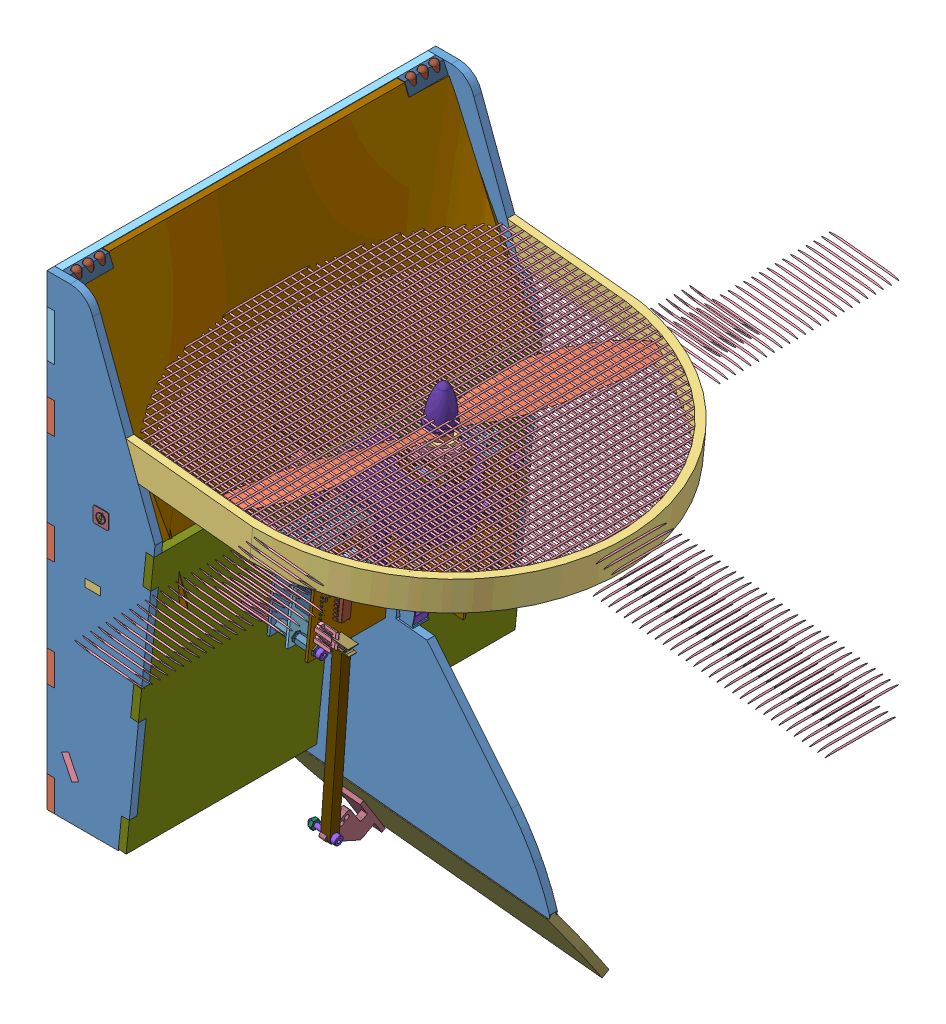
SolidWorks assembly AssTotaleSimu5, configuration Défaut. Lengths in mm. (continued)
Components (placement in the parent): (continued)
- AssStructSimu-1: AssStructSimu [Défaut] at (-125.7658 -1.8483 624.6548) x (1 0 0) z (0 0 -1) size (253.25 324.59 251.6) (continued)
  - AssCarte-1: AssCarte [Défaut] at (38.0121 147.1029 290.772) x (-0.101852 0.9948 0) z (0.9948 0.101852 0) size (66.52 130.57 98.72) (continued)
    - carte_onduleur_v3-1: carte_onduleur_v3 [Défaut] at (-131.8199 12.0892 20.7912) size (66.52 130.57 82.34) (continued)
      - U_DSPIC-1: U_DSPIC [Défaut] at (1.863 -2.61 0.803) size (7.92 35.56 7.75)
        - Open CASCADE STEP translator 6.8 1.17.1-1: Open CASCADE STEP translator 6.8 1.17.1 [Défaut] at origin size (7.92 35.56 7.75)
          - Body_1_4-1: Body_1_4 [Défaut] at (0 -0.2 4) x (1 0 0) z (0 -1 0) size (7.92 7.75 35.56)
      - C_DEC_DSPIC-1: C_DEC_DSPIC [Défaut] at (7.7 -8.8 -0.803) x (0 1 0) z (0 0 -1) size (2.34 1.04 0.5)
        - Open CASCADE STEP translator 6.8 1.6.1-1: Open CASCADE STEP translator 6.8 1.6.1 [Défaut] at origin size (2.34 1.04 0.5)
          - Body_1-1: Body_1 [Défaut] at origin size (2.29 1.04 0.43)
          - Pin_1-1: Pin_1 [Défaut] at (0.3048 0 0) x (-1 0 0) z (0 0 1) size (0.51 1.02 0.5)
          - Pin_2-1: Pin_2 [Défaut] at origin size (0.51 1.02 0.5)
      - IN-1: IN [Défaut] at (24.3 -5.3 0.803) x (0 1 0) z (0 0 1) size (10.21 15.56 26.9)
        - Open CASCADE STEP translator 6.8 1.19.1-1: Open CASCADE STEP translator 6.8 1.19.1 [Défaut] at origin size (10.21 15.56 26.9)
          - Body_1_3-1: Body_1_3 [Défaut] at (-13.5 1.8 3) x (0 1 0) z (1 0 0) size (15.56 26.9 10.21)
            - Imported-1: Imported [Défaut] at (2.0451 -4.5908 20.9802) size (8.6 15.9 10.16)
            - Imported-2: Imported [Défaut] at (-1.6683 9.1092 15.9802) x (0 0 1) z (-1 0 0) size (10.1 18.2 15.1)
              - Imported_2-1: Imported_2 [Défaut] at origin size (10.1 18.2 15.1)
              - Imported_3-1: Imported_3 [Défaut] at origin size (3.43 12.4 4.99)
              - Imported_4-1: Imported_4 [Défaut] at origin size (3.43 12.4 4.99)
              - Imported_5-1: Imported_5 [Défaut] at origin size (3.9 4.9 7)
              - Imported_6-1: Imported_6 [Défaut] at origin size (3.9 4.9 7)
              - Imported_7-1: Imported_7 [Défaut] at origin size (3.8 3.8 6.92)
              - Imported_8-1: Imported_8 [Défaut] at origin size (3.8 3.8 6.92)
              - Imported_9-1: Imported_9 [Défaut] at origin size (9 2.4 14.2)
      - CARTE_CMD-1: CARTE_CMD [Défaut] at (25 57.2 0.803) size (60.1 130 26.71)
        - Open CASCADE STEP translator 6.8 1.20.1-1: Open CASCADE STEP translator 6.8 1.20.1 [Défaut] at origin size (60.1 130 26.71)
          - Body_1_4-1: Body_1_4 [Défaut] at (-55 5 12) size (60.1 130 26.71)
            - 1_2-1: 1_2 [Défaut] at origin size (60.1 130 1.61)
            - 4-1: 4 [Défaut] at (23.6 -124.9 0.803) x (0 1 0) z (0 0 1) size (5 15.24 14.3)
              - =_[0_1_1_4]_2-1: =_[0_1_1_4]_2 [Défaut] at origin size (5 15.24 14.3)
                - 5-1: 5 [Défaut] at (0 -6.5 -13) x (0 1 0) z (0 0 -1) size (15.24 5 14.3)
            - 7-1: 7 [Défaut] at (23.6 -5 0.803) x (0 1 0) z (0 0 1) size (5 15.24 14.3)
              - =_[0_1_1_7]-1: =_[0_1_1_7] [Défaut] at origin size (5 15.24 14.3)
                - 5-1: 5 [Défaut] at (0 -6.5 -13) x (0 1 0) z (0 0 -1) size (15.24 5 14.3)
            - 10_2-1: 10_2 [Défaut] at (18.4 -115.6 0.803) size (25.4 7.92 7.75)
              - =_[0_1_1_9]-1: =_[0_1_1_9] [Défaut] at origin size (25.4 7.92 7.75)
                - 8-1: 8 [Défaut] at (11.2 4 0) x (0 1 0) z (1 0 0) size (7.92 7.75 25.4)
            - 13_2-1: 13_2 [Défaut] at (55.4 -114.7 0.803) x (-1 0 0) z (0 0 1) size (5 7.62 14.3)
              - =_[0_1_1_12]-1: =_[0_1_1_12] [Défaut] at origin size (5 7.62 14.3)
                - 11-1: 11 [Défaut] at (0 -2.5 11) x (0 -1 0) z (0 0 1) size (7.62 5 14.3)
            - 25-1: 25 [Défaut] at (56.9 -12.8 0.803) x (-1 0 0) z (0 0 1) size (16.02 47.26 11.05)
              - =_[0_1_1_15]_2-1: =_[0_1_1_15]_2 [Défaut] at origin size (16.02 47.26 11.05)
                - 23-1: 23 [Défaut] at (-36.5 21 4) x (0 -1 0) z (1 0 0) size (47.26 11.05 16.02)
                  - 14-1: 14 [Défaut] at (-7.4961 -1.5352 42.5833) size (42.58 6.55 16.01)
                  - 22-1: 22 [Défaut] at (19.3039 2.3748 37.905) x (-1 0 0) z (0 0 -1) size (10.36 6.14 15.24)
                    - 21-1: 21 [Défaut] at origin size (10.36 6.14 7.62)
                      - 19_2-1: 19_2 [Défaut] at origin size (10.36 6.14 2.54)
                        - 15-1: 15 [Défaut] at origin size (8.4 2.54 2.54)
                        - 16-1: 16 [Défaut] at (-0.0461 1.2682 1.27) x (0 0 -1) z (0.999998 -0.002105 0) size (1.95 5.07 7.58)
                      - 19_2-2: 19_2 [Défaut] at (0 0 -2.54) size (10.36 6.14 2.54)
                        - 15-1: 15 [Défaut] at origin size (8.4 2.54 2.54)
                        - 16-1: 16 [Défaut] at (-0.0461 1.2682 1.27) x (0 0 -1) z (0.999998 -0.002105 0) size (1.95 5.07 7.58)
                      - 19_2-3: 19_2 [Défaut] at (0 0 -5.08) size (10.36 6.14 2.54)
                        - 15-1: 15 [Défaut] at origin size (8.4 2.54 2.54)
                        - 16-1: 16 [Défaut] at (-0.0461 1.2682 1.27) x (0 0 -1) z (0.999998 -0.002105 0) size (1.95 5.07 7.58)
                    - 21-2: 21 [Défaut] at (0 0 -7.62) size (10.36 6.14 7.62)
                      - 19_2-1: 19_2 [Défaut] at origin size (10.36 6.14 2.54)
                        - 15-1: 15 [Défaut] at origin size (8.4 2.54 2.54)
                        - 16-1: 16 [Défaut] at (-0.0461 1.2682 1.27) x (0 0 -1) z (0.999998 -0.002105 0) size (1.95 5.07 7.58)
                      - 19_2-2: 19_2 [Défaut] at (0 0 -2.54) size (10.36 6.14 2.54)
                        - 15-1: 15 [Défaut] at origin size (8.4 2.54 2.54)
                        - 16-1: 16 [Défaut] at (-0.0461 1.2682 1.27) x (0 0 -1) z (0.999998 -0.002105 0) size (1.95 5.07 7.58)
                      - 19_2-3: 19_2 [Défaut] at (0 0 -5.08) size (10.36 6.14 2.54)
                        - 15-1: 15 [Défaut] at origin size (8.4 2.54 2.54)
                        - 16-1: 16 [Défaut] at (-0.0461 1.2682 1.27) x (0 0 -1) z (0.999998 -0.002105 0) size (1.95 5.07 7.58)
            - 31-1: 31 [Défaut] at (12.9 -104.5 0.803) size (6.76 3.64 4.37)
              - =_[0_1_1_24]-1: =_[0_1_1_24] [Défaut] at origin size (6.76 3.64 4.37)
                - 29-1: 29 [Défaut] at (-0.3 -2 0) size (6.76 3.64 4.37)
                  - =_[0_1_1_3]_3-1: =_[0_1_1_3]_3 [Défaut] at origin size (6 3.64 4.37)
                  - =_[0_1_1_4]_3-1: =_[0_1_1_4]_3 [Défaut] at origin size (0.38 1 0.67)
                  - =_[0_1_1_5]_3-1: =_[0_1_1_5]_3 [Défaut] at origin size (0.38 1 0.67)
            - 36-1: 36 [Défaut] at (28.6 -12.2 0.803) x (0 -1 0) z (0 0 1) size (2.34 1.04 0.5)
              - =_[0_1_1_30]-1: =_[0_1_1_30] [Défaut] at origin size (2.34 1.04 0.5)
                - 32_2-1: 32_2 [Défaut] at origin size (2.29 1.04 0.43)
                - 33_2-1: 33_2 [Défaut] at (0.3048 0 0) x (-1 0 0) z (0 0 1) size (0.51 1.02 0.5)
                - 34-1: 34 [Défaut] at origin size (0.51 1.02 0.5)
            - 38-1: 38 [Défaut] at (23.7 -12.2 0.803) x (0 -1 0) z (0 0 1) size (2.34 1.04 0.5)
              - =_[0_1_1_30]-1: =_[0_1_1_30] [Défaut] at origin size (2.34 1.04 0.5)
                - 32_2-1: 32_2 [Défaut] at origin size (2.29 1.04 0.43)
                - 33_2-1: 33_2 [Défaut] at (0.3048 0 0) x (-1 0 0) z (0 0 1) size (0.51 1.02 0.5)
                - 34-1: 34 [Défaut] at origin size (0.51 1.02 0.5)
            - 40_2-1: 40_2 [Défaut] at (26.2 -12.2 0.803) x (0 -1 0) z (0 0 1) size (2.34 1.04 0.5)
              - =_[0_1_1_30]-1: =_[0_1_1_30] [Défaut] at origin size (2.34 1.04 0.5)
                - 32_2-1: 32_2 [Défaut] at origin size (2.29 1.04 0.43)
                - 33_2-1: 33_2 [Défaut] at (0.3048 0 0) x (-1 0 0) z (0 0 1) size (0.51 1.02 0.5)
                - 34-1: 34 [Défaut] at origin size (0.51 1.02 0.5)
            - 42_2-1: 42_2 [Défaut] at (24.4 -119.2 0.803) size (2.34 1.04 0.5)
              - =_[0_1_1_30]-1: =_[0_1_1_30] [Défaut] at origin size (2.34 1.04 0.5)
                - 32_2-1: 32_2 [Défaut] at origin size (2.29 1.04 0.43)
                - 33_2-1: 33_2 [Défaut] at (0.3048 0 0) x (-1 0 0) z (0 0 1) size (0.51 1.02 0.5)
                - 34-1: 34 [Défaut] at origin size (0.51 1.02 0.5)
            - 45-1: 45 [Défaut] at (46.4 -125 0.803) size (5.08 5 14.3)
              - =_[0_1_1_38]-1: =_[0_1_1_38] [Défaut] at origin size (5.08 5 14.3)
                - 46-1: 46 [Défaut] at (1.2 0 11) size (5.08 5 14.3)
            - 48-1: 48 [Défaut] at (40.1 -125 0.803) size (5.08 5 14.3)
              - =_[0_1_1_41]-1: =_[0_1_1_41] [Défaut] at origin size (5.08 5 14.3)
                - 46-1: 46 [Défaut] at (1.2 0 11) size (5.08 5 14.3)
            - 51-1: 51 [Défaut] at (6.4 -119.9 0.803) x (0 1 0) z (0 0 1) size (15.24 2.54 7.37)
              - =_[0_1_1_43]-1: =_[0_1_1_43] [Défaut] at origin size (15.24 2.54 7.37)
                - 49_2-1: 49_2 [Défaut] at (6.5 0 0) x (1 0 0) z (0 -1 0) size (15.24 7.37 2.54)
            - 57_2-1: 57_2 [Défaut] at (50.8796 -121.1 -0.803) x (-1 0 0) z (0 0 -1) size (2.54 1.98 0.64)
              - =_[0_1_1_46]-1: =_[0_1_1_46] [Défaut] at origin size (2.54 1.98 0.64)
                - 52-1: 52 [Défaut] at origin size (2.54 1.14 0.58)
                - 53-1: 53 [Défaut] x (0 -1 0) z (0 0 1) size (0.43 0.51 0.38)
                - 54-1: 54 [Défaut] at (1.8796 1.8796 0) x (0 -1 0) z (0 0 1) size (0.43 0.51 0.38)
                - 55-1: 55 [Défaut] at (-0.9652 -2.8448 0) x (0 1 0) z (0 0 1) size (0.41 0.51 0.38)
            - 59_2-1: 59_2 [Défaut] at (43.6398 -120.995 -0.803) x (-1 0 0) z (0 0 -1) size (2.54 1.98 0.64)
              - =_[0_1_1_46]-1: =_[0_1_1_46] [Défaut] at origin size (2.54 1.98 0.64)
                - 52-1: 52 [Défaut] at origin size (2.54 1.14 0.58)
                - 53-1: 53 [Défaut] x (0 -1 0) z (0 0 1) size (0.43 0.51 0.38)
                - 54-1: 54 [Défaut] at (1.8796 1.8796 0) x (0 -1 0) z (0 0 1) size (0.43 0.51 0.38)
                - 55-1: 55 [Défaut] at (-0.9652 -2.8448 0) x (0 1 0) z (0 0 1) size (0.41 0.51 0.38)
            - 61_2-1: 61_2 [Défaut] at (47.6 -119.9 -0.803) x (-1 0 0) z (0 0 -1) size (2.34 1.04 0.5)
              - =_[0_1_1_30]-1: =_[0_1_1_30] [Défaut] at origin size (2.34 1.04 0.5)
                - 32_2-1: 32_2 [Défaut] at origin size (2.29 1.04 0.43)
                - 33_2-1: 33_2 [Défaut] at (0.3048 0 0) x (-1 0 0) z (0 0 1) size (0.51 1.02 0.5)
                - 34-1: 34 [Défaut] at origin size (0.51 1.02 0.5)
            - 63-1: 63 [Défaut] at (40.4 -119.9 -0.803) x (-1 0 0) z (0 0 -1) size (2.34 1.04 0.5)
              - =_[0_1_1_30]-1: =_[0_1_1_30] [Défaut] at origin size (2.34 1.04 0.5)
                - 32_2-1: 32_2 [Défaut] at origin size (2.29 1.04 0.43)
                - 33_2-1: 33_2 [Défaut] at (0.3048 0 0) x (-1 0 0) z (0 0 1) size (0.51 1.02 0.5)
                - 34-1: 34 [Défaut] at origin size (0.51 1.02 0.5)
            - 68-1: 68 [Défaut] at (47.7 -21.8 -0.803) x (0 1 0) z (0 0 -1) size (2.34 1.04 0.5)
              - =_[0_1_1_55]-1: =_[0_1_1_55] [Défaut] at origin size (2.34 1.04 0.5)
                - 64-1: 64 [Défaut] at origin size (2.29 1.04 0.43)
                - 65-1: 65 [Défaut] at (0.3048 0 0) x (-1 0 0) z (0 0 1) size (0.51 1.02 0.5)
                - 66-1: 66 [Défaut] at origin size (0.51 1.02 0.5)
            - 70-1: 70 [Défaut] at (47.6 -121.7 -0.803) x (-1 0 0) z (0 0 -1) size (2.34 1.04 0.5)
              - =_[0_1_1_30]-1: =_[0_1_1_30] [Défaut] at origin size (2.34 1.04 0.5)
                - 32_2-1: 32_2 [Défaut] at origin size (2.29 1.04 0.43)
                - 33_2-1: 33_2 [Défaut] at (0.3048 0 0) x (-1 0 0) z (0 0 1) size (0.51 1.02 0.5)
                - 34-1: 34 [Défaut] at origin size (0.51 1.02 0.5)
            - 72_2-1: 72_2 [Défaut] at (40.4 -121.5 -0.803) x (-1 0 0) z (0 0 -1) size (2.34 1.04 0.5)
              - =_[0_1_1_30]-1: =_[0_1_1_30] [Défaut] at origin size (2.34 1.04 0.5)
                - 32_2-1: 32_2 [Défaut] at origin size (2.29 1.04 0.43)
                - 33_2-1: 33_2 [Défaut] at (0.3048 0 0) x (-1 0 0) z (0 0 1) size (0.51 1.02 0.5)
                - 34-1: 34 [Défaut] at origin size (0.51 1.02 0.5)
            - 74_2-1: 74_2 [Défaut] at (47.7 -18.3 -0.803) x (0 1 0) z (0 0 -1) size (2.34 1.04 0.5)
              - =_[0_1_1_55]-1: =_[0_1_1_55] [Défaut] at origin size (2.34 1.04 0.5)
                - 64-1: 64 [Défaut] at origin size (2.29 1.04 0.43)
                - 65-1: 65 [Défaut] at (0.3048 0 0) x (-1 0 0) z (0 0 1) size (0.51 1.02 0.5)
                - 66-1: 66 [Défaut] at origin size (0.51 1.02 0.5)
            - 76_2-1: 76_2 [Défaut] at (45.5 -118.3 -0.803) x (1 0 0) z (0 0 -1) size (2.34 1.04 0.5)
              - =_[0_1_1_30]-1: =_[0_1_1_30] [Défaut] at origin size (2.34 1.04 0.5)
                - 32_2-1: 32_2 [Défaut] at origin size (2.29 1.04 0.43)
                - 33_2-1: 33_2 [Défaut] at (0.3048 0 0) x (-1 0 0) z (0 0 1) size (0.51 1.02 0.5)
                - 34-1: 34 [Défaut] at origin size (0.51 1.02 0.5)
            - 78_2-1: 78_2 [Défaut] at (38.2 -118.3 -0.803) x (1 0 0) z (0 0 -1) size (2.34 1.04 0.5)
              - =_[0_1_1_30]-1: =_[0_1_1_30] [Défaut] at origin size (2.34 1.04 0.5)
                - 32_2-1: 32_2 [Défaut] at origin size (2.29 1.04 0.43)
                - 33_2-1: 33_2 [Défaut] at (0.3048 0 0) x (-1 0 0) z (0 0 1) size (0.51 1.02 0.5)
                - 34-1: 34 [Défaut] at origin size (0.51 1.02 0.5)
            - 80_2-1: 80_2 [Défaut] at (28.6 -10.7 0.803) x (0 1 0) z (0 0 1) size (2.34 1.04 0.5)
              - =_[0_1_1_55]-1: =_[0_1_1_55] [Défaut] at origin size (2.34 1.04 0.5)
                - 64-1: 64 [Défaut] at origin size (2.29 1.04 0.43)
                - 65-1: 65 [Défaut] at (0.3048 0 0) x (-1 0 0) z (0 0 1) size (0.51 1.02 0.5)
                - 66-1: 66 [Défaut] at origin size (0.51 1.02 0.5)
            - 82_2-1: 82_2 [Défaut] at (23.7 -10.7 0.803) x (0 1 0) z (0 0 1) size (2.34 1.04 0.5)
              - =_[0_1_1_55]-1: =_[0_1_1_55] [Défaut] at origin size (2.34 1.04 0.5)
                - 64-1: 64 [Défaut] at origin size (2.29 1.04 0.43)
                - 65-1: 65 [Défaut] at (0.3048 0 0) x (-1 0 0) z (0 0 1) size (0.51 1.02 0.5)
                - 66-1: 66 [Défaut] at origin size (0.51 1.02 0.5)
            - 84-1: 84 [Défaut] at (26.2 -10.7 0.803) x (0 1 0) z (0 0 1) size (2.34 1.04 0.5)
              - =_[0_1_1_55]-1: =_[0_1_1_55] [Défaut] at origin size (2.34 1.04 0.5)
                - 64-1: 64 [Défaut] at origin size (2.29 1.04 0.43)
                - 65-1: 65 [Défaut] at (0.3048 0 0) x (-1 0 0) z (0 0 1) size (0.51 1.02 0.5)
                - 66-1: 66 [Défaut] at origin size (0.51 1.02 0.5)
            - 86-1: 86 [Défaut] at (23.0336 -119.2 0.803) x (-1 0 0) z (0 0 1) size (2.34 1.04 0.5)
              - =_[0_1_1_55]-1: =_[0_1_1_55] [Défaut] at origin size (2.34 1.04 0.5)
                - 64-1: 64 [Défaut] at origin size (2.29 1.04 0.43)
                - 65-1: 65 [Défaut] at (0.3048 0 0) x (-1 0 0) z (0 0 1) size (0.51 1.02 0.5)
                - 66-1: 66 [Défaut] at origin size (0.51 1.02 0.5)
            - 88-1: 88 [Défaut] at (14.1 -114.2 0.803) x (0 -1 0) z (0 0 1) size (2.34 1.04 0.5)
              - =_[0_1_1_55]-1: =_[0_1_1_55] [Défaut] at origin size (2.34 1.04 0.5)
                - 64-1: 64 [Défaut] at origin size (2.29 1.04 0.43)
                - 65-1: 65 [Défaut] at (0.3048 0 0) x (-1 0 0) z (0 0 1) size (0.51 1.02 0.5)
                - 66-1: 66 [Défaut] at origin size (0.51 1.02 0.5)
            - 90-1: 90 [Défaut] at (43.6 -107.8 -0.803) x (1 0 0) z (0 0 -1) size (2.34 1.04 0.5)
              - =_[0_1_1_55]-1: =_[0_1_1_55] [Défaut] at origin size (2.34 1.04 0.5)
                - 64-1: 64 [Défaut] at origin size (2.29 1.04 0.43)
                - 65-1: 65 [Défaut] at (0.3048 0 0) x (-1 0 0) z (0 0 1) size (0.51 1.02 0.5)
                - 66-1: 66 [Défaut] at origin size (0.51 1.02 0.5)
            - 92-1: 92 [Défaut] at (43.6 -106 -0.803) x (1 0 0) z (0 0 -1) size (2.34 1.04 0.5)
              - =_[0_1_1_55]-1: =_[0_1_1_55] [Défaut] at origin size (2.34 1.04 0.5)
                - 64-1: 64 [Défaut] at origin size (2.29 1.04 0.43)
                - 65-1: 65 [Défaut] at (0.3048 0 0) x (-1 0 0) z (0 0 1) size (0.51 1.02 0.5)
                - 66-1: 66 [Défaut] at origin size (0.51 1.02 0.5)
            - 175-1: 175 [Défaut] at (10 -21.7 0.803) x (0 -1 0) z (0 0 1) size (15 25.4 12.78)
              - =_[0_1_1_72]-1: =_[0_1_1_72] [Défaut] at origin size (15 25.4 12.78)
                - 173-1: 173 [Défaut] at (-1.4 -1 12) x (-1 0 0) z (0 1 0) size (15 12.78 25.4)
                  - board_1-1: board_1 [Défaut] at (-7.5 -1.57 12.5) size (15 1.57 25)
                  - hole_plating_20-1: hole_plating_20 [Défaut] at (-1.5 0 23.93) size (1.5 0.01 1.5)
                  - hole_plating_20-2: hole_plating_20 [Défaut] at (-1.5 0 21.39) size (1.5 0.01 1.5)
                  - hole_plating_20-3: hole_plating_20 [Défaut] at (-1.5 0 8.69) size (1.5 0.01 1.5)
                  - hole_plating_20-4: hole_plating_20 [Défaut] at (-1.5 -1.58 13.77) size (1.5 0.01 1.5)
                  - hole_plating_20-5: hole_plating_20 [Défaut] at (-1.5 0 16.31) size (1.5 0.01 1.5)
                  - hole_plating_20-6: hole_plating_20 [Défaut] at (-1.5 0 18.85) size (1.5 0.01 1.5)
                  - hole_plating_20-7: hole_plating_20 [Défaut] at (-1.5 0 13.77) size (1.5 0.01 1.5)
                  - hole_plating_20-8: hole_plating_20 [Défaut] at (-1.5 -1.58 11.23) size (1.5 0.01 1.5)
                  - hole_plating_20-9: hole_plating_20 [Défaut] at (-1.5 -1.58 18.85) size (1.5 0.01 1.5)
                  - hole_plating_20-10: hole_plating_20 [Défaut] at (-1.5 -1.58 6.15) size (1.5 0.01 1.5)
                  - hole_plating_20-11: hole_plating_20 [Défaut] at (-1.5 0 1.07) size (1.5 0.01 1.5)
                  - hole_plating_20-12: hole_plating_20 [Défaut] at (-1.5 -1.58 3.61) size (1.5 0.01 1.5)
                  - hole_plating_20-13: hole_plating_20 [Défaut] at (-1.5 -1.58 1.07) size (1.5 0.01 1.5)
                  - hole_plating_20-14: hole_plating_20 [Défaut] at (-1.5 -1.58 8.69) size (1.5 0.01 1.5)
                  - hole_plating_20-15: hole_plating_20 [Défaut] at (-1.5 -1.58 16.31) size (1.5 0.01 1.5)
                  - hole_plating_20-16: hole_plating_20 [Défaut] at (-1.5 0 11.23) size (1.5 0.01 1.5)
                  - hole_plating_20-17: hole_plating_20 [Défaut] at (-1.5 0 3.61) size (1.5 0.01 1.5)
                  - hole_plating_20-18: hole_plating_20 [Défaut] at (-1.5 -1.58 21.39) size (1.5 0.01 1.5)
                  - hole_plating_20-19: hole_plating_20 [Défaut] at (-1.5 0 6.15) size (1.5 0.01 1.5)
                  - hole_plating_20-20: hole_plating_20 [Défaut] at (-1.5 -1.58 23.93) size (1.5 0.01 1.5)
                  - Pin_Header_1x10_TH_Pitch_2.54mm_1-1: Pin_Header_1x10_TH_Pitch_2.54mm_1 [Défaut] at (-1.5 -1.5786 23.93) x (0 0 -1) z (0 -1 0) size (25.4 2.54 12.7)
                    - 124-1: 124 [Défaut] at origin size (25.4 2.54 2.8)
                      - =_[0_1_1_77]-1: =_[0_1_1_77] [Défaut] at origin size (2.54 2.54 2.8)
                      - =_[0_1_1_79]-1: =_[0_1_1_79] [Défaut] at origin size (2.54 2.54 2.8)
                      - =_[0_1_1_80]-1: =_[0_1_1_80] [Défaut] at origin size (2.54 2.54 2.8)
                      - =_[0_1_1_81]-1: =_[0_1_1_81] [Défaut] at origin size (2.54 2.54 2.8)
                      - =_[0_1_1_82]-1: =_[0_1_1_82] [Défaut] at origin size (2.54 2.54 2.8)
                      - =_[0_1_1_83]-1: =_[0_1_1_83] [Défaut] at origin size (2.54 2.54 2.8)
                      - =_[0_1_1_84]-1: =_[0_1_1_84] [Défaut] at origin size (2.54 2.54 2.8)
                      - =_[0_1_1_85]-1: =_[0_1_1_85] [Défaut] at origin size (2.54 2.54 2.8)
                      - =_[0_1_1_86]-1: =_[0_1_1_86] [Défaut] at origin size (2.54 2.54 2.8)
                      - =_[0_1_1_87]-1: =_[0_1_1_87] [Défaut] at origin size (2.54 2.54 2.8)
                    - 135-1: 135 [Défaut] at origin size (23.49 0.63 12.7)
                      - =_[0_1_1_88]-1: =_[0_1_1_88] [Défaut] at origin size (0.63 0.63 12.7)
                      - =_[0_1_1_90]-1: =_[0_1_1_90] [Défaut] at origin size (0.63 0.63 12.7)
                      - =_[0_1_1_91]-1: =_[0_1_1_91] [Défaut] at origin size (0.63 0.63 12.7)
                      - =_[0_1_1_92]-1: =_[0_1_1_92] [Défaut] at origin size (0.63 0.63 12.7)
                      - =_[0_1_1_93]-1: =_[0_1_1_93] [Défaut] at origin size (0.63 0.63 12.7)
                      - =_[0_1_1_94]-1: =_[0_1_1_94] [Défaut] at origin size (0.63 0.63 12.7)
                      - =_[0_1_1_95]-1: =_[0_1_1_95] [Défaut] at origin size (0.63 0.63 12.7)
                      - =_[0_1_1_96]-1: =_[0_1_1_96] [Défaut] at origin size (0.63 0.63 12.7)
                      - =_[0_1_1_97]-1: =_[0_1_1_97] [Défaut] at origin size (0.63 0.63 12.7)
                      - =_[0_1_1_98]-1: =_[0_1_1_98] [Défaut] at origin size (0.63 0.63 12.7)
                  - MPU-9250_1-1: MPU-9250_1 [Défaut] at (-8 0.05 12.5) x (-1 0 0) z (0 1 0) size (3 3 1.05)
                  - tantalum_10uF_1-1: tantalum_10uF_1 [Défaut] at (-13.167 0.1 10.9372) x (0 0 1) z (0 1 0) size (3.4 1.6 1.71)
                  - SOT23_5_1-1: SOT23_5_1 [Défaut] at (-7.475 -0.0136 21) x (0 0 1) z (0 1 0) size (3 3.2 0.92)
                  - RESC-0603_5-1: RESC-0603_5 [Défaut] at (-6.85 0 7.45) x (1 0 0) z (0 1 0) size (1.7 0.9 0.55)
                    - 143-1: 143 [Défaut] at origin size (1.7 0.9 0.55)
                      - =_[0_1_1_103]-1: =_[0_1_1_103] [Défaut] at origin size (0.4 0.9 0.53)
                      - =_[0_1_1_105]-1: =_[0_1_1_105] [Défaut] at origin size (0.4 0.9 0.53)
                      - =_[0_1_1_106]-1: =_[0_1_1_106] [Défaut] at origin size (1.64 0.9 0.52)
                    - 152-1: 152 [Défaut] at origin
                      - =_[0_1_1_107]-1: =_[0_1_1_107] [Défaut] at origin
                      - =_[0_1_1_109]-1: =_[0_1_1_109] [Défaut] at origin
                      - =_[0_1_1_110]-1: =_[0_1_1_110] [Défaut] at origin
                      - =_[0_1_1_111]-1: =_[0_1_1_111] [Défaut] at origin
                      - =_[0_1_1_112]-1: =_[0_1_1_112] [Défaut] at origin
                      - =_[0_1_1_113]-1: =_[0_1_1_113] [Défaut] at origin
                      - =_[0_1_1_114]-1: =_[0_1_1_114] [Défaut] at origin
                      - =_[0_1_1_115]-1: =_[0_1_1_115] [Défaut] at origin
                  - RESC-0603_5-2: RESC-0603_5 [Défaut] at (-9.85 0 16.05) x (1 0 0) z (0 1 0) size (1.7 0.9 0.55)
                    - 143-1: 143 [Défaut] at origin size (1.7 0.9 0.55)
                      - =_[0_1_1_103]-1: =_[0_1_1_103] [Défaut] at origin size (0.4 0.9 0.53)
                      - =_[0_1_1_105]-1: =_[0_1_1_105] [Défaut] at origin size (0.4 0.9 0.53)
                      - =_[0_1_1_106]-1: =_[0_1_1_106] [Défaut] at origin size (1.64 0.9 0.52)
                    - 152-1: 152 [Défaut] at origin
                      - =_[0_1_1_107]-1: =_[0_1_1_107] [Défaut] at origin
                      - =_[0_1_1_109]-1: =_[0_1_1_109] [Défaut] at origin
                      - =_[0_1_1_110]-1: =_[0_1_1_110] [Défaut] at origin
                      - =_[0_1_1_111]-1: =_[0_1_1_111] [Défaut] at origin
                      - =_[0_1_1_112]-1: =_[0_1_1_112] [Défaut] at origin
                      - =_[0_1_1_113]-1: =_[0_1_1_113] [Défaut] at origin
                      - =_[0_1_1_114]-1: =_[0_1_1_114] [Défaut] at origin
                      - =_[0_1_1_115]-1: =_[0_1_1_115] [Défaut] at origin
                  - RESC-0603_5-3: RESC-0603_5 [Défaut] at (-6.85 0 17.55) x (1 0 0) z (0 1 0) size (1.7 0.9 0.55)
                    - 143-1: 143 [Défaut] at origin size (1.7 0.9 0.55)
                      - =_[0_1_1_103]-1: =_[0_1_1_103] [Défaut] at origin size (0.4 0.9 0.53)
                      - =_[0_1_1_105]-1: =_[0_1_1_105] [Défaut] at origin size (0.4 0.9 0.53)
                      - =_[0_1_1_106]-1: =_[0_1_1_106] [Défaut] at origin size (1.64 0.9 0.52)
                    - 152-1: 152 [Défaut] at origin
                      - =_[0_1_1_107]-1: =_[0_1_1_107] [Défaut] at origin
                      - =_[0_1_1_109]-1: =_[0_1_1_109] [Défaut] at origin
                      - =_[0_1_1_110]-1: =_[0_1_1_110] [Défaut] at origin
                      - =_[0_1_1_111]-1: =_[0_1_1_111] [Défaut] at origin
                      - =_[0_1_1_112]-1: =_[0_1_1_112] [Défaut] at origin
                      - =_[0_1_1_113]-1: =_[0_1_1_113] [Défaut] at origin
                      - =_[0_1_1_114]-1: =_[0_1_1_114] [Défaut] at origin
                      - =_[0_1_1_115]-1: =_[0_1_1_115] [Défaut] at origin
                  - RESC-0603_5-4: RESC-0603_5 [Défaut] at (-6.85 0 16.05) x (1 0 0) z (0 1 0) size (1.7 0.9 0.55)
                    - 143-1: 143 [Défaut] at origin size (1.7 0.9 0.55)
                      - =_[0_1_1_103]-1: =_[0_1_1_103] [Défaut] at origin size (0.4 0.9 0.53)
                      - =_[0_1_1_105]-1: =_[0_1_1_105] [Défaut] at origin size (0.4 0.9 0.53)
                      - =_[0_1_1_106]-1: =_[0_1_1_106] [Défaut] at origin size (1.64 0.9 0.52)
                    - 152-1: 152 [Défaut] at origin
                      - =_[0_1_1_107]-1: =_[0_1_1_107] [Défaut] at origin
                      - =_[0_1_1_109]-1: =_[0_1_1_109] [Défaut] at origin
                      - =_[0_1_1_110]-1: =_[0_1_1_110] [Défaut] at origin
                      - =_[0_1_1_111]-1: =_[0_1_1_111] [Défaut] at origin
                      - =_[0_1_1_112]-1: =_[0_1_1_112] [Défaut] at origin
                      - =_[0_1_1_113]-1: =_[0_1_1_113] [Défaut] at origin
                      - =_[0_1_1_114]-1: =_[0_1_1_114] [Défaut] at origin
                      - =_[0_1_1_115]-1: =_[0_1_1_115] [Défaut] at origin
                  - RESC-0603_5-5: RESC-0603_5 [Défaut] at (-6.85 0 5.95) x (1 0 0) z (0 1 0) size (1.7 0.9 0.55)
                    - 143-1: 143 [Défaut] at origin size (1.7 0.9 0.55)
                      - =_[0_1_1_103]-1: =_[0_1_1_103] [Défaut] at origin size (0.4 0.9 0.53)
                      - =_[0_1_1_105]-1: =_[0_1_1_105] [Défaut] at origin size (0.4 0.9 0.53)
                      - =_[0_1_1_106]-1: =_[0_1_1_106] [Défaut] at origin size (1.64 0.9 0.52)
                    - 152-1: 152 [Défaut] at origin
                      - =_[0_1_1_107]-1: =_[0_1_1_107] [Défaut] at origin
                      - =_[0_1_1_109]-1: =_[0_1_1_109] [Défaut] at origin
                      - =_[0_1_1_110]-1: =_[0_1_1_110] [Défaut] at origin
                      - =_[0_1_1_111]-1: =_[0_1_1_111] [Défaut] at origin
                      - =_[0_1_1_112]-1: =_[0_1_1_112] [Défaut] at origin
                      - =_[0_1_1_113]-1: =_[0_1_1_113] [Défaut] at origin
                      - =_[0_1_1_114]-1: =_[0_1_1_114] [Défaut] at origin
                      - =_[0_1_1_115]-1: =_[0_1_1_115] [Défaut] at origin
                  - CAPC-0603-T0.9-BN_5-1: CAPC-0603-T0.9-BN_5 [Défaut] at (-9.85 0 8.95) x (1 0 0) z (0 1 0) size (1.7 0.9 0.9)
                    - =_[0_1_1_117]-1: =_[0_1_1_117] [Défaut] at origin size (1.7 0.9 0.9)
                    - 167-1: 167 [Défaut] at origin
                      - =_[0_1_1_118]-1: =_[0_1_1_118] [Défaut] at origin
                      - =_[0_1_1_120]-1: =_[0_1_1_120] [Défaut] at origin
                      - =_[0_1_1_121]-1: =_[0_1_1_121] [Défaut] at origin
                      - =_[0_1_1_122]-1: =_[0_1_1_122] [Défaut] at origin
                      - =_[0_1_1_123]-1: =_[0_1_1_123] [Défaut] at origin
                      - =_[0_1_1_124]-1: =_[0_1_1_124] [Défaut] at origin
                      - =_[0_1_1_125]-1: =_[0_1_1_125] [Défaut] at origin
                      - =_[0_1_1_126]-1: =_[0_1_1_126] [Défaut] at origin
                  - CAPC-0603-T0.9-BN_5-2: CAPC-0603-T0.9-BN_5 [Défaut] at (-6.85 0 8.95) x (1 0 0) z (0 1 0) size (1.7 0.9 0.9)
                    - =_[0_1_1_117]-1: =_[0_1_1_117] [Défaut] at origin size (1.7 0.9 0.9)
                    - 167-1: 167 [Défaut] at origin
                      - =_[0_1_1_118]-1: =_[0_1_1_118] [Défaut] at origin
                      - =_[0_1_1_120]-1: =_[0_1_1_120] [Défaut] at origin
                      - =_[0_1_1_121]-1: =_[0_1_1_121] [Défaut] at origin
                      - =_[0_1_1_122]-1: =_[0_1_1_122] [Défaut] at origin
                      - =_[0_1_1_123]-1: =_[0_1_1_123] [Défaut] at origin
                      - =_[0_1_1_124]-1: =_[0_1_1_124] [Défaut] at origin
                      - =_[0_1_1_125]-1: =_[0_1_1_125] [Défaut] at origin
                      - =_[0_1_1_126]-1: =_[0_1_1_126] [Défaut] at origin
                  - CAPC-0603-T0.9-BN_5-3: CAPC-0603-T0.9-BN_5 [Défaut] at (-6.85 0 19.05) x (1 0 0) z (0 1 0) size (1.7 0.9 0.9)
                    - =_[0_1_1_117]-1: =_[0_1_1_117] [Défaut] at origin size (1.7 0.9 0.9)
                    - 167-1: 167 [Défaut] at origin
                      - =_[0_1_1_118]-1: =_[0_1_1_118] [Défaut] at origin
                      - =_[0_1_1_120]-1: =_[0_1_1_120] [Défaut] at origin
                      - =_[0_1_1_121]-1: =_[0_1_1_121] [Défaut] at origin
                      - =_[0_1_1_122]-1: =_[0_1_1_122] [Défaut] at origin
                      - =_[0_1_1_123]-1: =_[0_1_1_123] [Défaut] at origin
                      - =_[0_1_1_124]-1: =_[0_1_1_124] [Défaut] at origin
                      - =_[0_1_1_125]-1: =_[0_1_1_125] [Défaut] at origin
                      - =_[0_1_1_126]-1: =_[0_1_1_126] [Défaut] at origin
                  - CAPC-0603-T0.9-BN_5-4: CAPC-0603-T0.9-BN_5 [Défaut] at (-9.85 0 7.45) x (1 0 0) z (0 1 0) size (1.7 0.9 0.9)
                    - =_[0_1_1_117]-1: =_[0_1_1_117] [Défaut] at origin size (1.7 0.9 0.9)
                    - 167-1: 167 [Défaut] at origin
                      - =_[0_1_1_118]-1: =_[0_1_1_118] [Défaut] at origin
                      - =_[0_1_1_120]-1: =_[0_1_1_120] [Défaut] at origin
                      - =_[0_1_1_121]-1: =_[0_1_1_121] [Défaut] at origin
                      - =_[0_1_1_122]-1: =_[0_1_1_122] [Défaut] at origin
                      - =_[0_1_1_123]-1: =_[0_1_1_123] [Défaut] at origin
                      - =_[0_1_1_124]-1: =_[0_1_1_124] [Défaut] at origin
                      - =_[0_1_1_125]-1: =_[0_1_1_125] [Défaut] at origin
                      - =_[0_1_1_126]-1: =_[0_1_1_126] [Défaut] at origin
                  - CAPC-0603-T0.9-BN_5-5: CAPC-0603-T0.9-BN_5 [Défaut] at (-9.85 0 17.55) x (1 0 0) z (0 1 0) size (1.7 0.9 0.9)
                    - =_[0_1_1_117]-1: =_[0_1_1_117] [Défaut] at origin size (1.7 0.9 0.9)
                    - 167-1: 167 [Défaut] at origin
                      - =_[0_1_1_118]-1: =_[0_1_1_118] [Défaut] at origin
                      - =_[0_1_1_120]-1: =_[0_1_1_120] [Défaut] at origin
                      - =_[0_1_1_121]-1: =_[0_1_1_121] [Défaut] at origin
                      - =_[0_1_1_122]-1: =_[0_1_1_122] [Défaut] at origin
                      - =_[0_1_1_123]-1: =_[0_1_1_123] [Défaut] at origin
                      - =_[0_1_1_124]-1: =_[0_1_1_124] [Défaut] at origin
                      - =_[0_1_1_125]-1: =_[0_1_1_125] [Défaut] at origin
                      - =_[0_1_1_126]-1: =_[0_1_1_126] [Défaut] at origin
            - 177-1: 177 [Défaut] at (52.1 -16.5 -0.803) x (1 0 0) z (0 0 -1) size (2.34 1.04 0.5)
              - =_[0_1_1_30]-1: =_[0_1_1_30] [Défaut] at origin size (2.34 1.04 0.5)
                - 32_2-1: 32_2 [Défaut] at origin size (2.29 1.04 0.43)
                - 33_2-1: 33_2 [Défaut] at (0.3048 0 0) x (-1 0 0) z (0 0 1) size (0.51 1.02 0.5)
                - 34-1: 34 [Défaut] at origin size (0.51 1.02 0.5)
            - 179-1: 179 [Défaut] at (22.5336 -121.5 -0.803) x (-1 0 0) z (0 0 -1) size (2.34 1.04 0.5)
              - =_[0_1_1_30]-1: =_[0_1_1_30] [Défaut] at origin size (2.34 1.04 0.5)
                - 32_2-1: 32_2 [Défaut] at origin size (2.29 1.04 0.43)
                - 33_2-1: 33_2 [Défaut] at (0.3048 0 0) x (-1 0 0) z (0 0 1) size (0.51 1.02 0.5)
                - 34-1: 34 [Défaut] at origin size (0.51 1.02 0.5)
            - 181-1: 181 [Défaut] at (48.6 -127 -0.803) x (-1 0 0) z (0 0 -1) size (2.34 1.04 0.5)
              - =_[0_1_1_30]-1: =_[0_1_1_30] [Défaut] at origin size (2.34 1.04 0.5)
                - 32_2-1: 32_2 [Défaut] at origin size (2.29 1.04 0.43)
                - 33_2-1: 33_2 [Défaut] at (0.3048 0 0) x (-1 0 0) z (0 0 1) size (0.51 1.02 0.5)
                - 34-1: 34 [Défaut] at origin size (0.51 1.02 0.5)
            - 183-1: 183 [Défaut] at (26.0189 -121.5 0.803) size (2.34 1.04 0.5)
              - =_[0_1_1_30]-1: =_[0_1_1_30] [Défaut] at origin size (2.34 1.04 0.5)
                - 32_2-1: 32_2 [Défaut] at origin size (2.29 1.04 0.43)
                - 33_2-1: 33_2 [Défaut] at (0.3048 0 0) x (-1 0 0) z (0 0 1) size (0.51 1.02 0.5)
                - 34-1: 34 [Défaut] at origin size (0.51 1.02 0.5)
            - 185-1: 185 [Défaut] at (30.3664 -19 -0.803) x (1 0 0) z (0 0 -1) size (2.34 1.04 0.5)
              - =_[0_1_1_30]-1: =_[0_1_1_30] [Défaut] at origin size (2.34 1.04 0.5)
                - 32_2-1: 32_2 [Défaut] at origin size (2.29 1.04 0.43)
                - 33_2-1: 33_2 [Défaut] at (0.3048 0 0) x (-1 0 0) z (0 0 1) size (0.51 1.02 0.5)
                - 34-1: 34 [Défaut] at origin size (0.51 1.02 0.5)
            - 187-1: 187 [Défaut] at (51.7 -114.3 -0.803) x (0 1 0) z (0 0 -1) size (2.34 1.04 0.5)
              - =_[0_1_1_30]-1: =_[0_1_1_30] [Défaut] at origin size (2.34 1.04 0.5)
                - 32_2-1: 32_2 [Défaut] at origin size (2.29 1.04 0.43)
                - 33_2-1: 33_2 [Défaut] at (0.3048 0 0) x (-1 0 0) z (0 0 1) size (0.51 1.02 0.5)
                - 34-1: 34 [Défaut] at origin size (0.51 1.02 0.5)
            - 189-1: 189 [Défaut] at (50 -114.3 -0.803) x (0 1 0) z (0 0 -1) size (2.34 1.04 0.5)
              - =_[0_1_1_30]-1: =_[0_1_1_30] [Défaut] at origin size (2.34 1.04 0.5)
                - 32_2-1: 32_2 [Défaut] at origin size (2.29 1.04 0.43)
                - 33_2-1: 33_2 [Défaut] at (0.3048 0 0) x (-1 0 0) z (0 0 1) size (0.51 1.02 0.5)
                - 34-1: 34 [Défaut] at origin size (0.51 1.02 0.5)
      - C2_1-1: C2_1 [Défaut] at (-20.6984 1.8 -0.803) x (1 0 0) z (0 0 -1) size (2.34 1.04 0.5)
        - Open CASCADE STEP translator 6.8 1.6.1-1: Open CASCADE STEP translator 6.8 1.6.1 [Défaut] at origin size (2.34 1.04 0.5)
          - Body_1-1: Body_1 [Défaut] at origin size (2.29 1.04 0.43)
          - Pin_1-1: Pin_1 [Défaut] at (0.3048 0 0) x (-1 0 0) z (0 0 1) size (0.51 1.02 0.5)
          - Pin_2-1: Pin_2 [Défaut] at origin size (0.51 1.02 0.5)
      - C2_2-1: C2_2 [Défaut] at (-24.2 1.8 -0.803) x (1 0 0) z (0 0 -1) size (2.34 1.04 0.5)
        - Open CASCADE STEP translator 6.8 1.6.1-1: Open CASCADE STEP translator 6.8 1.6.1 [Défaut] at origin size (2.34 1.04 0.5)
          - Body_1-1: Body_1 [Défaut] at origin size (2.29 1.04 0.43)
          - Pin_1-1: Pin_1 [Défaut] at (0.3048 0 0) x (-1 0 0) z (0 0 1) size (0.51 1.02 0.5)
          - Pin_2-1: Pin_2 [Défaut] at origin size (0.51 1.02 0.5)
      - C3_1-1: C3_1 [Défaut] at (-20.9176 -12.8 -0.803) x (1 0 0) z (0 0 -1) size (2.34 1.04 0.5)
        - Open CASCADE STEP translator 6.8 1.6.1-1: Open CASCADE STEP translator 6.8 1.6.1 [Défaut] at origin size (2.34 1.04 0.5)
          - Body_1-1: Body_1 [Défaut] at origin size (2.29 1.04 0.43)
          - Pin_1-1: Pin_1 [Défaut] at (0.3048 0 0) x (-1 0 0) z (0 0 1) size (0.51 1.02 0.5)
          - Pin_2-1: Pin_2 [Défaut] at origin size (0.51 1.02 0.5)
      - C3_2-1: C3_2 [Défaut] at (-24.4 -12.8 -0.803) x (1 0 0) z (0 0 -1) size (2.34 1.04 0.5)
        - Open CASCADE STEP translator 6.8 1.6.1-1: Open CASCADE STEP translator 6.8 1.6.1 [Défaut] at origin size (2.34 1.04 0.5)
          - Body_1-1: Body_1 [Défaut] at origin size (2.29 1.04 0.43)
          - Pin_1-1: Pin_1 [Défaut] at (0.3048 0 0) x (-1 0 0) z (0 0 1) size (0.51 1.02 0.5)
          - Pin_2-1: Pin_2 [Défaut] at origin size (0.51 1.02 0.5)
      - D_CUR-1: D_CUR [Défaut] at (-12.4432 3.85 -0.803) x (0 -1 0) z (0 0 -1) size (2.7 5.2 1.11)
        - Open CASCADE STEP translator 6.8 1.25.1-1: Open CASCADE STEP translator 6.8 1.25.1 [Défaut] at origin size (2.7 5.2 1.11)
          - Body_1_5-1: Body_1_5 [Défaut] at (1.2 -4 0) x (0 1 0) z (0 0 1) size (5.2 2.7 1.11)
            - =_[0_1_1_3]_4-1: =_[0_1_1_3]_4 [Défaut] at origin size (0.39 0.64 0.01)
            - =_[0_1_1_4]_4-1: =_[0_1_1_4]_4 [Défaut] at origin size (0.6 1.9 0.2)
            - =_[0_1_1_5]_4-1: =_[0_1_1_5]_4 [Défaut] at origin size (0.21 0.08 0.01)
            - =_[0_1_1_6]_2-1: =_[0_1_1_6]_2 [Défaut] at origin size (0.6 1.9 0.2)
            - =_[0_1_1_7]_2-1: =_[0_1_1_7]_2 [Défaut] at origin size (0.46 0.68 0.01)
            - =_[0_1_1_8]_2-1: =_[0_1_1_8]_2 [Défaut] at origin size (0.38 0.66 0.01)
            - =_[0_1_1_9]-1: =_[0_1_1_9] [Défaut] at origin size (0.2 0.62 0.01)
            - =_[0_1_1_10]-1: =_[0_1_1_10] [Défaut] at origin size (4 2.7 1.1)
            - =_[0_1_1_11]-1: =_[0_1_1_11] [Défaut] at origin size (0.46 0.63 0.01)
            - =_[0_1_1_12]-1: =_[0_1_1_12] [Défaut] at origin size (0.56 0.68 0.01)
      - RC1_1-1: RC1_1 [Défaut] at (-20.7176 8.1 -0.803) x (1 0 0) z (0 0 -1) size (2.34 1.04 0.5)
        - Open CASCADE STEP translator 6.8 1.12.1-1: Open CASCADE STEP translator 6.8 1.12.1 [Défaut] at origin size (2.34 1.04 0.5)
          - Body_1_3-1: Body_1_3 [Défaut] at origin size (2.29 1.04 0.43)
          - Pin_1_2-1: Pin_1_2 [Défaut] at (0.3048 0 0) x (-1 0 0) z (0 0 1) size (0.51 1.02 0.5)
          - Pin_2_2-1: Pin_2_2 [Défaut] at origin size (0.51 1.02 0.5)
      - RC1_2-1: RC1_2 [Défaut] at (-22 8.1 -0.803) x (-1 0 0) z (0 0 -1) size (2.34 1.04 0.5)
        - Open CASCADE STEP translator 6.8 1.12.1-1: Open CASCADE STEP translator 6.8 1.12.1 [Défaut] at origin size (2.34 1.04 0.5)
          - Body_1_3-1: Body_1_3 [Défaut] at origin size (2.29 1.04 0.43)
          - Pin_1_2-1: Pin_1_2 [Défaut] at (0.3048 0 0) x (-1 0 0) z (0 0 1) size (0.51 1.02 0.5)
          - Pin_2_2-1: Pin_2_2 [Défaut] at origin size (0.51 1.02 0.5)
      - RC2_1-1: RC2_1 [Défaut] at (-20.716 0.243 -0.803) x (1 0 0) z (0 0 -1) size (2.34 1.04 0.5)
        - Open CASCADE STEP translator 6.8 1.12.1-1: Open CASCADE STEP translator 6.8 1.12.1 [Défaut] at origin size (2.34 1.04 0.5)
          - Body_1_3-1: Body_1_3 [Défaut] at origin size (2.29 1.04 0.43)
          - Pin_1_2-1: Pin_1_2 [Défaut] at (0.3048 0 0) x (-1 0 0) z (0 0 1) size (0.51 1.02 0.5)
          - Pin_2_2-1: Pin_2_2 [Défaut] at origin size (0.51 1.02 0.5)
      - RC2_2-1: RC2_2 [Défaut] at (-22 0.18 -0.803) x (-1 0 0) z (0 0 -1) size (2.34 1.04 0.5)
        - Open CASCADE STEP translator 6.8 1.12.1-1: Open CASCADE STEP translator 6.8 1.12.1 [Défaut] at origin size (2.34 1.04 0.5)
          - Body_1_3-1: Body_1_3 [Défaut] at origin size (2.29 1.04 0.43)
          - Pin_1_2-1: Pin_1_2 [Défaut] at (0.3048 0 0) x (-1 0 0) z (0 0 1) size (0.51 1.02 0.5)
